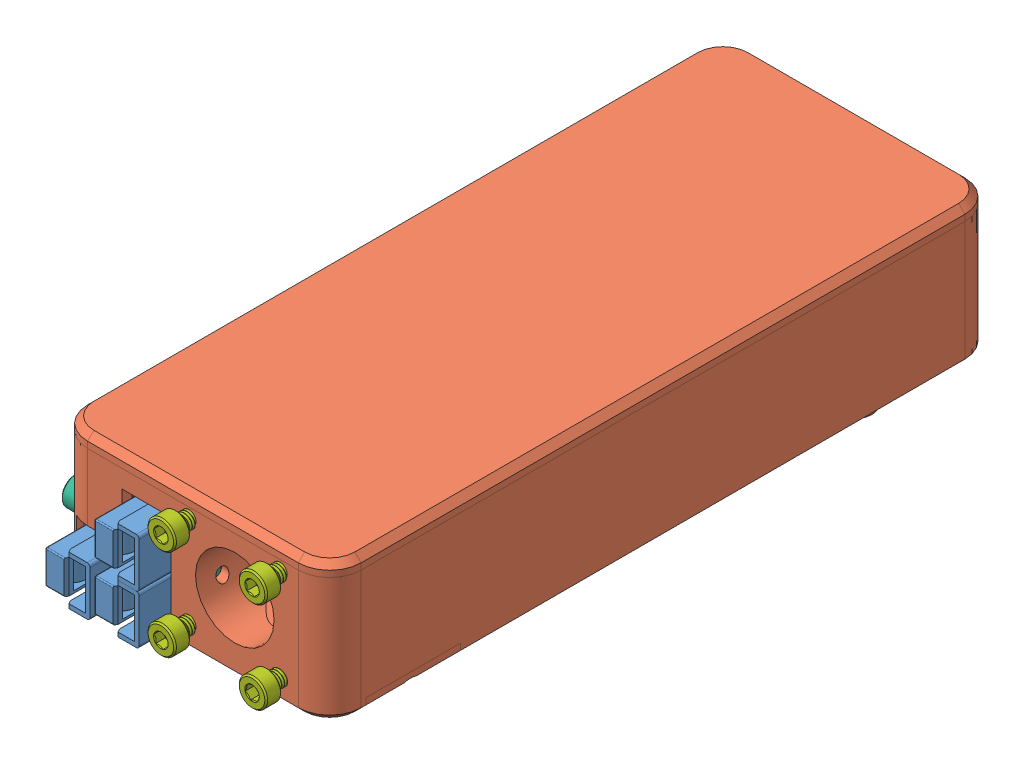
SolidWorks assembly AxxSolder_Portable, configuration Default. Lengths in mm.
Overall size (44.62 37.3 111.1).
17 component instances, 7 part files, 27 mates.
Components (placement in the parent):
- Anderson_PowerPole-3: Anderson_PowerPole [Default] at (-7.3715 3.9141 34.4539) x (0 -1 0) z (0 0 1) size (16.24 16.24 22.71)
  - powerpole 15-45A housing.step-3: powerpole 15-45A housing.step [Default] at origin size (8.44 8.44 22.71)
  - powerpole 15-45A housing.step-5: powerpole 15-45A housing.step [Default] at (-7.8 0 0) size (8.44 8.44 22.71)
  - powerpole 15-45A housing.step-6: powerpole 15-45A housing.step [Default] at (0 -7.8 0) size (8.44 8.44 22.71)
- Encolsure_Portable-1: Encolsure_Portable [Default] at origin size (43.5 21.95 106)
- AxxSolder-2: AxxSolder [Default] at (19.48 8 -50.802) x (1 0 0) z (0 -1 0) size (39.06 82.54 35.41)
- 92703A451_18-8 Stainless Steel Torx Flat Head Screws-1: 92703A451_18-8 Stainless Steel Torx Flat Head Screws [92703A451] at (-15.24 -1.455 29.2) x (1 0 0) z (0 -1 0) size (4.7 4.7 12.12)
- 90236A105_Zinc-Plated Steel Torx Flat Head Screws-1: 90236A105_Zinc-Plated Steel Torx Flat Head Screws [90236A105] at (16.35 -1.3849 34.7) x (1 0 0) z (0 -1 0) size (3.8 3.8 8.15)
- 91292A019_18-8 Stainless Steel Socket Head Screw-1: 91292A019_18-8 Stainless Steel Socket Head Screw [91292A019] at (-0.25 7.8 49) x (0 -0.459877 -0.887983) z (1 0 0) size (4.5 4.5 22.72)
- 91292A010_18-8 Stainless Steel Socket Head Screw-1: 91292A010_18-8 Stainless Steel Socket Head Screw [91292A010] at (13.9 2.35 49) x (0.705565 0.708645 0) z (0 0 -1) size (4.5 4.5 8.64)
- 92703A451_18-8 Stainless Steel Torx Flat Head Screws-2: 92703A451_18-8 Stainless Steel Torx Flat Head Screws [92703A451] at (15.24 -1.455 29.2) x (1 0 0) z (0 -1 0) size (4.7 4.7 12.12)
- 92703A451_18-8 Stainless Steel Torx Flat Head Screws-3: 92703A451_18-8 Stainless Steel Torx Flat Head Screws [92703A451] at (16.5 -1.455 -47.75) x (1 0 0) z (0 -1 0) size (4.7 4.7 12.12)
- 92703A451_18-8 Stainless Steel Torx Flat Head Screws-4: 92703A451_18-8 Stainless Steel Torx Flat Head Screws [92703A451] at (-16.5 -1.455 -47.75) x (1 0 0) z (0 -1 0) size (4.7 4.7 12.12)
- 90236A105_Zinc-Plated Steel Torx Flat Head Screws-2: 90236A105_Zinc-Plated Steel Torx Flat Head Screws [90236A105] at (16.35 -1.3849 44.7) x (1 0 0) z (0 -1 0) size (3.8 3.8 8.15)
- 91292A010_18-8 Stainless Steel Socket Head Screw-2: 91292A010_18-8 Stainless Steel Socket Head Screw [91292A010] at (-0.6 2.35 49) x (-0.251051 -0.967974 0) z (0 0 -1) size (4.5 4.5 8.64)
- 91292A010_18-8 Stainless Steel Socket Head Screw-3: 91292A010_18-8 Stainless Steel Socket Head Screw [91292A010] at (13.9 16.85 49) x (-0.251051 -0.967974 0) z (0 0 -1) size (4.5 4.5 8.64)
- 91292A010_18-8 Stainless Steel Socket Head Screw-4: 91292A010_18-8 Stainless Steel Socket Head Screw [91292A010] at (-0.6 16.85 49) x (-0.251051 -0.967974 0) z (0 0 -1) size (4.5 4.5 8.64)
Mates (geometry in assembly coordinates):
- Coincident1: coincident aligned: plane of Encolsure_Portable-1 through (0 0 0) normal (0 0 1)
- Coincident2: coincident aligned: plane of Encolsure_Portable-1 through (0 0 0) normal (0 1 0)
- Coincident3: coincident aligned: plane of Encolsure_Portable-1 through (0 0 0) normal (1 0 0)
- Coincident4: coincident anti-aligned: plane of Encolsure_Portable-1 through (-15.24 8 29.2) normal (0 -1 0); plane of AxxSolder-2 through (-0.02 8 -9.552) normal (0 1 0)
- Concentric1: concentric anti-aligned: cylinder of Encolsure_Portable-1 through (-15.24 8 29.2) axis (0 1 0) radius 1.05; cylinder of AxxSolder-2 through (-15.24 8.01 29.2) axis (0 -1 0) radius 1.25
- Concentric2: concentric anti-aligned: cylinder of Encolsure_Portable-1 through (15.24 8 29.2) axis (0 1 0) radius 1.05; cylinder of AxxSolder-2 through (15.24 8.01 29.2) axis (0 -1 0) radius 1.25
- Coincident11: coincident anti-aligned: plane of Anderson_PowerPole-3/powerpole 15-45A housing.step-3 through (-3.45 7.8 58.1) normal (1 0 0); plane of Encolsure_Portable-1 through (-3.45 0 56.5) normal (-1 0 0)
- Coincident12: coincident anti-aligned: plane of Anderson_PowerPole-3/powerpole 15-45A housing.step-3 through (-3.45 0 58.1) normal (0 -1 0); plane of Encolsure_Portable-1 through (-16.75 0 48) normal (0 1 0)
- Distance1: distance = 5.1 mm aligned: plane of Anderson_PowerPole-3/powerpole 15-45A housing.step-3 through (-11.25 7.8 58.1) normal (0 0 1); plane of Encolsure_Portable-1 through (-16.75 -1.5 53) normal (0 0 1)
- Width1: width anti-aligned: plane of Mini Rocker 4-Pin Switch-1 through (-7.25 1.788 33.85) normal (0 0 -1); plane of Mini Rocker 4-Pin Switch-1 through (-7.25 1.788 51.35) normal (0 0 1); plane of Encolsure_Portable-1 through (-29.75 14.3 32.7) normal (0 0 1); plane of Encolsure_Portable-1 through (-29.75 14.3 52.5) normal (0 0 -1)
- Coincident13: coincident anti-aligned: plane of Encolsure_Portable-1 through (-21.75 -1.5 -48) normal (-1 0 0); plane of Mini Rocker 4-Pin Switch-1 through (-21.75 8.238 42.6) normal (1 0 0)
- Coincident14: coincident aligned: cone of Encolsure_Portable-1 through (-15.24 -1.5 29.2) axis (0 1 0); cone of 92703A451_18-8 Stainless Steel Torx Flat Head Screws-1 through (-15.24 0.045 29.2) axis (0 1 0)
- Coincident15: coincident aligned: cone of Encolsure_Portable-1 through (16.35 -1.5 34.7) axis (0 1 0); cone of 90236A105_Zinc-Plated Steel Torx Flat Head Screws-1 through (16.35 -0.1849 34.7) axis (0 1 0)
- Concentric3: concentric anti-aligned: cylinder of Encolsure_Portable-1 through (-20.25 7.8 49) axis (-1 0 0) radius 2.325; cylinder of 91292A019_18-8 Stainless Steel Socket Head Screw-1 through (-22.75 7.8 49) axis (1 0 0) radius 2.25
- Coincident16: coincident anti-aligned: plane of Encolsure_Portable-1 through (-20.25 7.8 49) normal (-1 0 0); plane of 91292A019_18-8 Stainless Steel Socket Head Screw-1 through (-20.25 7.8 49) normal (1 0 0)
- Concentric4: concentric aligned: cylinder of Encolsure_Portable-1 through (13.9 2.35 56.5) axis (0 0 -1) radius 1; cylinder of 91292A010_18-8 Stainless Steel Socket Head Screw-1 through (13.9 2.35 57.5) axis (0 0 -1) radius 2.25
- Coincident18: coincident aligned: cone of Encolsure_Portable-1 through (15.24 -1.5 29.2) axis (0 1 0); cone of 92703A451_18-8 Stainless Steel Torx Flat Head Screws-2 through (15.24 0.045 29.2) axis (0 1 0)
- Coincident19: coincident aligned: cone of Encolsure_Portable-1 through (16.5 -1.5 -47.75) axis (0 1 0); cone of 92703A451_18-8 Stainless Steel Torx Flat Head Screws-3 through (16.5 0.045 -47.75) axis (0 1 0)
- Coincident20: coincident aligned: cone of Encolsure_Portable-1 through (-16.5 -1.5 -47.75) axis (0 1 0); cone of 92703A451_18-8 Stainless Steel Torx Flat Head Screws-4 through (-16.5 0.045 -47.75) axis (0 1 0)
- Coincident21: coincident aligned: cone of Encolsure_Portable-1 through (16.35 -1.5 44.7) axis (0 1 0); cone of 90236A105_Zinc-Plated Steel Torx Flat Head Screws-2 through (16.35 -0.1849 44.7) axis (0 1 0)
- Coincident22: coincident aligned: plane of 91292A010_18-8 Stainless Steel Socket Head Screw-1 through (13.9 2.35 57.5) normal (0 0 1); plane of 91292A010_18-8 Stainless Steel Socket Head Screw-2 through (-0.6 2.35 57.5) normal (0 0 1)
- Coincident23: coincident aligned: plane of 91292A010_18-8 Stainless Steel Socket Head Screw-2 through (-0.6 2.35 57.5) normal (0 0 1); plane of 91292A010_18-8 Stainless Steel Socket Head Screw-3 through (13.9 16.85 57.5) normal (0 0 1)
- Coincident24: coincident aligned: plane of 91292A010_18-8 Stainless Steel Socket Head Screw-3 through (13.9 16.85 57.5) normal (0 0 1); plane of 91292A010_18-8 Stainless Steel Socket Head Screw-4 through (-0.6 16.85 57.5) normal (0 0 1)
- Concentric5: concentric aligned: cylinder of 91292A010_18-8 Stainless Steel Socket Head Screw-4 through (-0.6 16.85 57.5) axis (0 0 -1) radius 2.25; cylinder of Encolsure_Portable-1 through (-0.6 16.85 56.5) axis (0 0 -1) radius 1
- Concentric6: concentric aligned: cylinder of Encolsure_Portable-1 through (-0.6 2.35 56.5) axis (0 0 -1) radius 1; cylinder of 91292A010_18-8 Stainless Steel Socket Head Screw-2 through (-0.6 2.35 57.5) axis (0 0 -1) radius 2.25
- Concentric7: concentric aligned: cylinder of Encolsure_Portable-1 through (13.9 16.85 56.5) axis (0 0 -1) radius 1; cylinder of 91292A010_18-8 Stainless Steel Socket Head Screw-3 through (13.9 16.85 57.5) axis (0 0 -1) radius 2.25
- Distance2: distance = 2 mm anti-aligned: plane of Encolsure_Portable-1 through (-16.75 -1.5 53) normal (0 0 1); plane of 91292A010_18-8 Stainless Steel Socket Head Screw-1 through (13.9 2.35 55) normal (0 0 -1)
